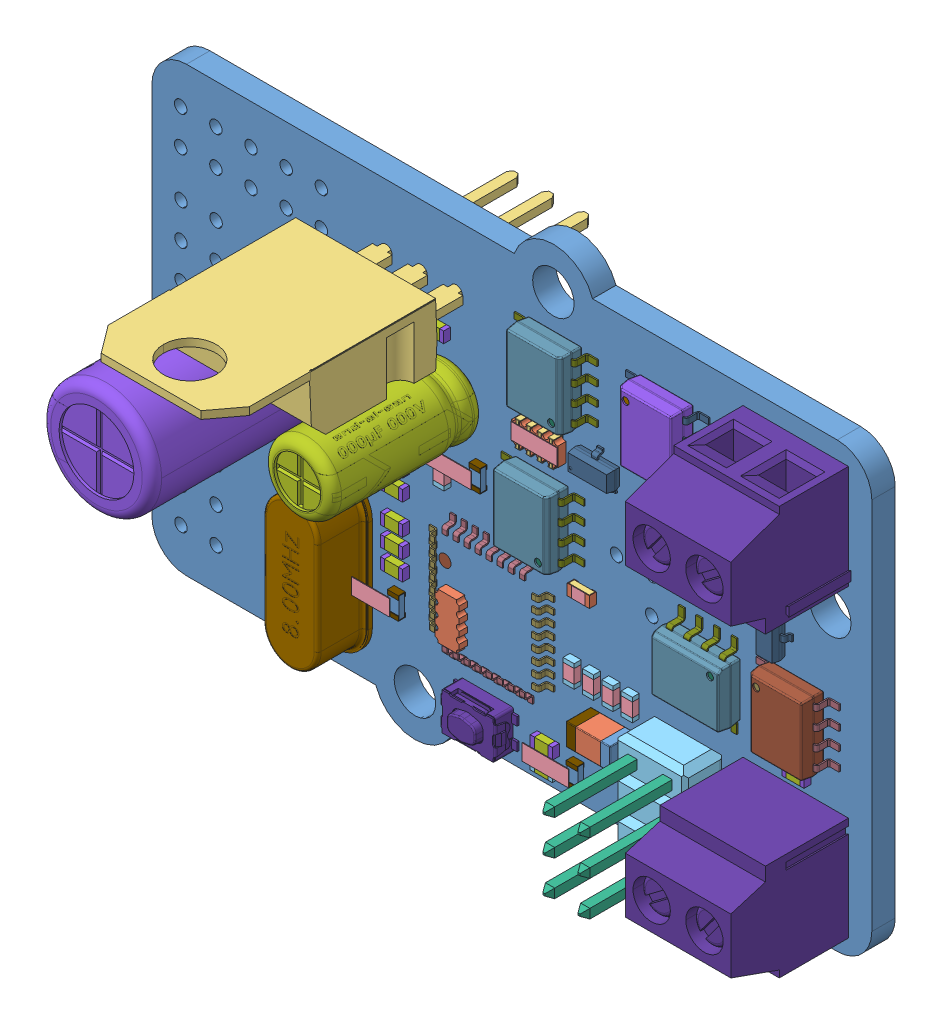
SolidWorks assembly DMotor_PCB v2.8, configuration По умолчанию. Lengths in mm.
Overall size (52 36 28.9).
344 component instances, 44 part files, 0 mates.
Components (placement in the parent):
- DMotor_PCB v2.8.step-1: DMotor_PCB v2.8.step [По умолчанию] at origin size (52 36 28.9)
  - Board.step-1: Board.step [По умолчанию] at origin size (52 36 1.69)
    - Open CASCADE STEP translator 6.8 1.1.1.step-1: Open CASCADE STEP translator 6.8 1.1.1.step [По умолчанию] at (0 0 -1.692) size (52 36 1.69)
  - RN1.step-1: RN1.step [По умолчанию] at origin size (3.35 1.85 0.7)
    - 5778449216.step-1: 5778449216.step [По умолчанию] at (28.3 21.5 0) x (0 1 0) z (0 0 1) size (1.85 3.35 0.7)
      - body.step-1: body.step [По умолчанию] at (-0.875 -1.675 0) size (1.75 3.35 0.6)
        - Open_CASCADE_STEP_translator_6.8_25.1.1.step-1: Open_CASCADE_STEP_translator_6.8_25.1.1.step [По умолчанию] at origin size (1.75 3.35 0.6)
      - Mid_Pin.step-1: Mid_Pin.step [По умолчанию] at (-0.875 -1.2 0) size (0.3 0.38 0.7)
        - Open_CASCADE_STEP_translator_6.8_25.3.1.step-1: Open_CASCADE_STEP_translator_6.8_25.3.1.step [По умолчанию] at origin size (0.3 0.38 0.7)
      - Mid_Pin.step-2: Mid_Pin.step [По умолчанию] at (0.875 1.2 0) x (-1 0 0) z (0 0 1) size (0.3 0.38 0.7)
        - Open_CASCADE_STEP_translator_6.8_25.3.1.step-1: Open_CASCADE_STEP_translator_6.8_25.3.1.step [По умолчанию] at origin size (0.3 0.38 0.7)
      - Mid_Pin.step-3: Mid_Pin.step [По умолчанию] at (-0.875 -0.4 0) size (0.3 0.38 0.7)
        - Open_CASCADE_STEP_translator_6.8_25.3.1.step-1: Open_CASCADE_STEP_translator_6.8_25.3.1.step [По умолчанию] at origin size (0.3 0.38 0.7)
      - Mid_Pin.step-4: Mid_Pin.step [По умолчанию] at (0.875 0.4 0) x (-1 0 0) z (0 0 1) size (0.3 0.38 0.7)
        - Open_CASCADE_STEP_translator_6.8_25.3.1.step-1: Open_CASCADE_STEP_translator_6.8_25.3.1.step [По умолчанию] at origin size (0.3 0.38 0.7)
      - Mid_Pin.step-5: Mid_Pin.step [По умолчанию] at (-0.875 0.4 0) size (0.3 0.38 0.7)
        - Open_CASCADE_STEP_translator_6.8_25.3.1.step-1: Open_CASCADE_STEP_translator_6.8_25.3.1.step [По умолчанию] at origin size (0.3 0.38 0.7)
      - Mid_Pin.step-6: Mid_Pin.step [По умолчанию] at (0.875 -0.4 0) x (-1 0 0) z (0 0 1) size (0.3 0.38 0.7)
        - Open_CASCADE_STEP_translator_6.8_25.3.1.step-1: Open_CASCADE_STEP_translator_6.8_25.3.1.step [По умолчанию] at origin size (0.3 0.38 0.7)
      - Mid_Pin.step-7: Mid_Pin.step [По умолчанию] at (-0.875 1.2 0) size (0.3 0.38 0.7)
        - Open_CASCADE_STEP_translator_6.8_25.3.1.step-1: Open_CASCADE_STEP_translator_6.8_25.3.1.step [По умолчанию] at origin size (0.3 0.38 0.7)
      - Mid_Pin.step-8: Mid_Pin.step [По умолчанию] at (0.875 -1.2 0) x (-1 0 0) z (0 0 1) size (0.3 0.38 0.7)
        - Open_CASCADE_STEP_translator_6.8_25.3.1.step-1: Open_CASCADE_STEP_translator_6.8_25.3.1.step [По умолчанию] at origin size (0.3 0.38 0.7)
      - mark.step-1: mark.step [По умолчанию] at (-0.875 -1.675 0) size (1.15 3.35 0.05)
  - ICSP.step-1: ICSP.step [По умолчанию] at origin size (5.08 7.62 12.7)
    - 2x3_TH_Pitch_2_54mm.step-1: 2x3_TH_Pitch_2_54mm.step [По умолчанию] at (38.7601 0.89 0) x (0 1 0) z (1 0 0) size (7.62 12.7 5.08)
      - header2x3.step-1: header2x3.step [По умолчанию] at (0 1.4 0) size (7.62 2.8 5.08)
      - pin.step-1: pin.step [По умолчанию] at (1.29 -3.5 1.29) size (0.67 12.7 0.67)
      - pin.step-2: pin.step [По умолчанию] at (1.29 -3.5 -1.25) size (0.67 12.7 0.67)
      - pin.step-3: pin.step [По умолчанию] at (3.83 -3.5 1.29) size (0.67 12.7 0.67)
      - pin.step-4: pin.step [По умолчанию] at (3.83 -3.5 -1.25) size (0.67 12.7 0.67)
      - pin.step-5: pin.step [По умолчанию] at (6.37 -3.5 1.29) size (0.67 12.7 0.67)
      - pin.step-6: pin.step [По умолчанию] at (6.37 -3.5 -1.25) size (0.67 12.7 0.67)
  - C9.step-1: C9.step [По умолчанию] at origin size (1.6 0.8 0.5)
    - 5928350752.step-1: 5928350752.step [По умолчанию] at (17.8 11.1 0) size (1 0.8 0.5)
      - Extruded.step-1: Extruded.step [По умолчанию] at origin size (1 0.8 0.5)
    - 5928351312.step-1: 5928351312.step [По умолчанию] at (18.45 11.1 0) size (0.3 0.8 0.5)
      - Extruded-0.step-1: Extruded-0.step [По умолчанию] at origin size (0.3 0.8 0.5)
    - 5928351312.step-2: 5928351312.step [По умолчанию] at (17.15 11.1 0) size (0.3 0.8 0.5)
      - Extruded-0.step-1: Extruded-0.step [По умолчанию] at origin size (0.3 0.8 0.5)
  - C11.step-1: C11.step [По умолчанию] at origin size (1.6 0.8 0.5)
    - 5928350752.step-1: 5928350752.step [По умолчанию] at (17.8 8.3 0) size (1 0.8 0.5)
      - Extruded.step-1: Extruded.step [По умолчанию] at origin size (1 0.8 0.5)
    - 5928351312.step-1: 5928351312.step [По умолчанию] at (18.45 8.3 0) size (0.3 0.8 0.5)
      - Extruded-0.step-1: Extruded-0.step [По умолчанию] at origin size (0.3 0.8 0.5)
    - 5928351312.step-2: 5928351312.step [По умолчанию] at (17.15 8.3 0) size (0.3 0.8 0.5)
      - Extruded-0.step-1: Extruded-0.step [По умолчанию] at origin size (0.3 0.8 0.5)
  - Y1.step-1: Y1.step [По умолчанию] at origin size (4.65 11.35 5.59)
    - HC-49S.step-1: HC-49S.step [По умолчанию] at (13.6 6.8251 0) x (0 1 0) z (1 0 0) size (11.35 5.59 4.65)
  - VT2.step-1: VT2.step [По умолчанию] at origin size (2.9 2.3 1)
    - SOT23-3.step-1: SOT23-3.step [По умолчанию] at (31 21.9 0) x (1 0 0) z (0 -1 0) size (2.9 1 2.3)
  - VT1.step-1: VT1.step [По умолчанию] at origin size (2.3 2.9 1)
    - SOT23-3.step-1: SOT23-3.step [По умолчанию] at (45.2 19.5 0) x (0 -1 0) z (-1 0 0) size (2.9 1 2.3)
  - U1.step-1: U1.step [По умолчанию] at origin size (9 9 1.11)
    - 5778452896.step-1: 5778452896.step [По умолчанию] at (24.6 9.05 0) size (9 9 1.11)
      - body.step-1: body.step [По умолчанию] at (-3.5 -3.5 0) size (1.75 3.35 0.6)
        - Open_CASCADE_STEP_translator_6.8_25.1.1.step-1: Open_CASCADE_STEP_translator_6.8_25.1.1.step [По умолчанию] at origin size (1.75 3.35 0.6)
      - Open_CASCADE_STEP_translator_6.8_22.1.step-1: Open_CASCADE_STEP_translator_6.8_22.1.step [По умолчанию] at (-3.5 -3.5 0.001) size (0.89 0.89 0.01)
      - Leader.step-1: Leader.step [По умолчанию] at (-3.5 -2.8 0) x (-1 0 0) z (0 0 1) size (1 0.38 0.68)
      - Leader.step-2: Leader.step [По умолчанию] at (-3.5 -2 0) x (-1 0 0) z (0 0 1) size (1 0.38 0.68)
      - Leader.step-3: Leader.step [По умолчанию] at (-3.5 -1.2 0) x (-1 0 0) z (0 0 1) size (1 0.38 0.68)
      - Leader.step-4: Leader.step [По умолчанию] at (-3.5 -0.4 0) x (-1 0 0) z (0 0 1) size (1 0.38 0.68)
      - Leader.step-5: Leader.step [По умолчанию] at (-3.5 0.4 0) x (-1 0 0) z (0 0 1) size (1 0.38 0.68)
      - Leader.step-6: Leader.step [По умолчанию] at (-3.5 1.2 0) x (-1 0 0) z (0 0 1) size (1 0.38 0.68)
      - Leader.step-7: Leader.step [По умолчанию] at (-3.5 2 0) x (-1 0 0) z (0 0 1) size (1 0.38 0.68)
      - Leader.step-8: Leader.step [По умолчанию] at (-3.5 2.8 0) x (-1 0 0) z (0 0 1) size (1 0.38 0.68)
      - Leader.step-9: Leader.step [По умолчанию] at (3.5 -2.8 0) size (1 0.38 0.68)
      - Leader.step-10: Leader.step [По умолчанию] at (3.5 -2 0) size (1 0.38 0.68)
      - Leader.step-11: Leader.step [По умолчанию] at (3.5 -1.2 0) size (1 0.38 0.68)
      - Leader.step-12: Leader.step [По умолчанию] at (3.5 -0.4 0) size (1 0.38 0.68)
      - Leader.step-13: Leader.step [По умолчанию] at (3.5 0.4 0) size (1 0.38 0.68)
      - Leader.step-14: Leader.step [По умолчанию] at (3.5 1.2 0) size (1 0.38 0.68)
      - Leader.step-15: Leader.step [По умолчанию] at (3.5 2 0) size (1 0.38 0.68)
      - Leader.step-16: Leader.step [По умолчанию] at (3.5 2.8 0) size (1 0.38 0.68)
      - Leader-1.step-1: Leader-1.step [По умолчанию] at (-2.8 -3.5 0) x (0 -1 0) z (0 0 1) size (1 0.38 0.68)
      - Leader-1.step-2: Leader-1.step [По умолчанию] at (-2 -3.5 0) x (0 -1 0) z (0 0 1) size (1 0.38 0.68)
      - Leader-1.step-3: Leader-1.step [По умолчанию] at (-1.2 -3.5 0) x (0 -1 0) z (0 0 1) size (1 0.38 0.68)
      - Leader-1.step-4: Leader-1.step [По умолчанию] at (-0.4 -3.5 0) x (0 -1 0) z (0 0 1) size (1 0.38 0.68)
      - Leader-1.step-5: Leader-1.step [По умолчанию] at (0.4 -3.5 0) x (0 -1 0) z (0 0 1) size (1 0.38 0.68)
      - Leader-1.step-6: Leader-1.step [По умолчанию] at (1.2 -3.5 0) x (0 -1 0) z (0 0 1) size (1 0.38 0.68)
      - Leader-1.step-7: Leader-1.step [По умолчанию] at (2 -3.5 0) x (0 -1 0) z (0 0 1) size (1 0.38 0.68)
      - Leader-1.step-8: Leader-1.step [По умолчанию] at (2.8 -3.5 0) x (0 -1 0) z (0 0 1) size (1 0.38 0.68)
      - Leader-1.step-9: Leader-1.step [По умолчанию] at (-2.8 3.5 0) x (0 1 0) z (0 0 1) size (1 0.38 0.68)
      - Leader-1.step-10: Leader-1.step [По умолчанию] at (-2 3.5 0) x (0 1 0) z (0 0 1) size (1 0.38 0.68)
      - Leader-1.step-11: Leader-1.step [По умолчанию] at (-1.2 3.5 0) x (0 1 0) z (0 0 1) size (1 0.38 0.68)
      - Leader-1.step-12: Leader-1.step [По умолчанию] at (-0.4 3.5 0) x (0 1 0) z (0 0 1) size (1 0.38 0.68)
      - Leader-1.step-13: Leader-1.step [По умолчанию] at (0.4 3.5 0) x (0 1 0) z (0 0 1) size (1 0.38 0.68)
      - Leader-1.step-14: Leader-1.step [По умолчанию] at (1.2 3.5 0) x (0 1 0) z (0 0 1) size (1 0.38 0.68)
      - Leader-1.step-15: Leader-1.step [По умолчанию] at (2 3.5 0) x (0 1 0) z (0 0 1) size (1 0.38 0.68)
      - Leader-1.step-16: Leader-1.step [По умолчанию] at (2.8 3.5 0) x (0 1 0) z (0 0 1) size (1 0.38 0.68)
  - U2.step-1: U2.step [По умолчанию] at origin size (6 5.01 1.75)
    - 5778448736.step-1: 5778448736.step [По умолчанию] at (28.3 17.1 0) x (-1 0 0) z (0 0 1) size (6 5 1.75)
      - Body-1.step-1: Body-1.step [По умолчанию] at (-2 -2.5 0) size (4 5 1.65)
        - Open_CASCADE_STEP_translator_6.8_4.2.1.step-1: Open_CASCADE_STEP_translator_6.8_4.2.1.step [По умолчанию] at origin size (4 5 1.65)
      - Open_CASCADE_STEP_translator_6.8_4.1.step-1: Open_CASCADE_STEP_translator_6.8_4.1.step [По умолчанию] at (-2 -2.5 0.001) size (0.51 0.51 0.01)
      - Leader-2.step-1: Leader-2.step [По умолчанию] at (-2 -1.905 0) x (-1 0 0) z (0 0 1) size (1 0.42 0.97)
      - Leader-2.step-2: Leader-2.step [По умолчанию] at (-2 -0.635 0) x (-1 0 0) z (0 0 1) size (1 0.42 0.97)
      - Leader-2.step-3: Leader-2.step [По умолчанию] at (-2 0.635 0) x (-1 0 0) z (0 0 1) size (1 0.42 0.97)
      - Leader-2.step-4: Leader-2.step [По умолчанию] at (-2 1.905 0) x (-1 0 0) z (0 0 1) size (1 0.42 0.97)
      - Leader-2.step-5: Leader-2.step [По умолчанию] at (2 -1.905 0) size (1 0.42 0.97)
      - Leader-2.step-6: Leader-2.step [По умолчанию] at (2 -0.635 0) size (1 0.42 0.97)
      - Leader-2.step-7: Leader-2.step [По умолчанию] at (2 0.635 0) size (1 0.42 0.97)
      - Leader-2.step-8: Leader-2.step [По умолчанию] at (2 1.905 0) size (1 0.42 0.97)
  - RESET.step-1: RESET.step [По умолчанию] at origin size (4.6 2.8 1.94)
    - KMR221GLFS.step-1: KMR221GLFS.step [По умолчанию] at (24.2249 2.1749 0) x (-1 0 0) z (0 1 0) size (4.6 1.94 2.8)
  - R7.step-1: R7.step [По умолчанию] at origin size (3.35 1.75 1.15)
    - 5778454576.step-1: 5778454576.step [По умолчанию] at (23.8 17 0) x (0 1 0) z (0 0 1) size (1.75 3.35 1.15)
      - Terminal.step-1: Terminal.step [По умолчанию] at (-0.8 -0.4 0) size (0.3 0.8 0.5)
        - Open_CASCADE_STEP_translator_6.8_7.2.1.step-1: Open_CASCADE_STEP_translator_6.8_7.2.1.step [По умолчанию] at origin size (0.3 0.8 0.5)
      - Terminal.step-2: Terminal.step [По умолчанию] at (0.8 0.4 0) x (-1 0 0) z (0 0 1) size (0.3 0.8 0.5)
        - Open_CASCADE_STEP_translator_6.8_7.2.1.step-1: Open_CASCADE_STEP_translator_6.8_7.2.1.step [По умолчанию] at origin size (0.3 0.8 0.5)
      - Mid_Body.step-1: Mid_Body.step [По умолчанию] at (-0.8 -0.4 0) size (1.5 0.8 0.4)
      - mark.step-1: mark.step [По умолчанию] at (-0.5 -0.4 0.45) size (1.15 3.35 0.05)
  - R6.step-1: R6.step [По умолчанию] at origin size (1.6 0.8 0.5)
    - 5778452416.step-1: 5778452416.step [По умолчанию] at (31.3 13.4 0) x (1 0 0) z (0 0 1) size (1.6 0.8 0.5)
      - Terminal-1.step-1: Terminal-1.step [По умолчанию] at (-0.8 -0.4 0) size (0.3 0.8 0.5)
        - Open_CASCADE_STEP_translator_6.8_7.2.1-3.step-1: Open_CASCADE_STEP_translator_6.8_7.2.1-3.step [По умолчанию] at origin size (0.3 0.8 0.5)
      - Terminal-1.step-2: Terminal-1.step [По умолчанию] at (0.8 0.4 0) x (-1 0 0) z (0 0 1) size (0.3 0.8 0.5)
        - Open_CASCADE_STEP_translator_6.8_7.2.1-3.step-1: Open_CASCADE_STEP_translator_6.8_7.2.1-3.step [По умолчанию] at origin size (0.3 0.8 0.5)
      - Mid_Body-4.step-1: Mid_Body-4.step [По умолчанию] at (-0.8 -0.4 0) size (1.5 0.8 0.4)
      - Mark-5.step-1: Mark-5.step [По умолчанию] at (-0.5 -0.4 0.45) size (1 0.8 0.05)
  - R5.step-1: R5.step [По умолчанию] at origin size (1.6 0.8 0.5)
    - 5778448016.step-1: 5778448016.step [По умолчанию] at (28.625 1.175 0) x (-1 0 0) z (0 0 1) size (1.6 0.8 0.5)
      - Terminal-2.step-1: Terminal-2.step [По умолчанию] at (-0.8 -0.4 0) size (0.3 0.8 0.5)
        - Open_CASCADE_STEP_translator_6.8_7.2.1-6.step-1: Open_CASCADE_STEP_translator_6.8_7.2.1-6.step [По умолчанию] at origin size (0.3 0.8 0.5)
      - Terminal-2.step-2: Terminal-2.step [По умолчанию] at (0.8 0.4 0) x (-1 0 0) z (0 0 1) size (0.3 0.8 0.5)
        - Open_CASCADE_STEP_translator_6.8_7.2.1-6.step-1: Open_CASCADE_STEP_translator_6.8_7.2.1-6.step [По умолчанию] at origin size (0.3 0.8 0.5)
      - Mid_Body-7.step-1: Mid_Body-7.step [По умолчанию] at (-0.8 -0.4 0) size (1.5 0.8 0.4)
      - Mark-8.step-1: Mark-8.step [По умолчанию] at (-0.5 -0.4 0.45) size (1 0.8 0.05)
  - R4.step-1: R4.step [По умолчанию] at origin size (3.35 1.75 1.15)
    - 5778454576.step-1: 5778454576.step [По умолчанию] at (30.825 1.875 0) x (0 1 0) z (0 0 1) size (1.75 3.35 1.15)
      - Terminal.step-1: Terminal.step [По умолчанию] at (-0.8 -0.4 0) size (0.3 0.8 0.5)
        - Open_CASCADE_STEP_translator_6.8_7.2.1.step-1: Open_CASCADE_STEP_translator_6.8_7.2.1.step [По умолчанию] at origin size (0.3 0.8 0.5)
      - Terminal.step-2: Terminal.step [По умолчанию] at (0.8 0.4 0) x (-1 0 0) z (0 0 1) size (0.3 0.8 0.5)
        - Open_CASCADE_STEP_translator_6.8_7.2.1.step-1: Open_CASCADE_STEP_translator_6.8_7.2.1.step [По умолчанию] at origin size (0.3 0.8 0.5)
      - Mid_Body.step-1: Mid_Body.step [По умолчанию] at (-0.8 -0.4 0) size (1.5 0.8 0.4)
      - mark.step-1: mark.step [По умолчанию] at (-0.5 -0.4 0.45) size (1.15 3.35 0.05)
  - R2.step-1: R2.step [По умолчанию] at origin size (3.35 1.75 1.15)
    - 5778454576.step-1: 5778454576.step [По умолчанию] at (10.025 13.8 0) x (0 1 0) z (0 0 1) size (1.75 3.35 1.15)
      - Terminal.step-1: Terminal.step [По умолчанию] at (-0.8 -0.4 0) size (0.3 0.8 0.5)
        - Open_CASCADE_STEP_translator_6.8_7.2.1.step-1: Open_CASCADE_STEP_translator_6.8_7.2.1.step [По умолчанию] at origin size (0.3 0.8 0.5)
      - Terminal.step-2: Terminal.step [По умолчанию] at (0.8 0.4 0) x (-1 0 0) z (0 0 1) size (0.3 0.8 0.5)
        - Open_CASCADE_STEP_translator_6.8_7.2.1.step-1: Open_CASCADE_STEP_translator_6.8_7.2.1.step [По умолчанию] at origin size (0.3 0.8 0.5)
      - Mid_Body.step-1: Mid_Body.step [По умолчанию] at (-0.8 -0.4 0) size (1.5 0.8 0.4)
      - mark.step-1: mark.step [По умолчанию] at (-0.5 -0.4 0.45) size (1.15 3.35 0.05)
  - R3.step-1: R3.step [По умолчанию] at origin size (3.35 1.75 1.15)
    - 5778454576.step-1: 5778454576.step [По умолчанию] at (17.9 6.1 0) x (0 1 0) z (0 0 1) size (1.75 3.35 1.15)
      - Terminal.step-1: Terminal.step [По умолчанию] at (-0.8 -0.4 0) size (0.3 0.8 0.5)
        - Open_CASCADE_STEP_translator_6.8_7.2.1.step-1: Open_CASCADE_STEP_translator_6.8_7.2.1.step [По умолчанию] at origin size (0.3 0.8 0.5)
      - Terminal.step-2: Terminal.step [По умолчанию] at (0.8 0.4 0) x (-1 0 0) z (0 0 1) size (0.3 0.8 0.5)
        - Open_CASCADE_STEP_translator_6.8_7.2.1.step-1: Open_CASCADE_STEP_translator_6.8_7.2.1.step [По умолчанию] at origin size (0.3 0.8 0.5)
      - Mid_Body.step-1: Mid_Body.step [По умолчанию] at (-0.8 -0.4 0) size (1.5 0.8 0.4)
      - mark.step-1: mark.step [По умолчанию] at (-0.5 -0.4 0.45) size (1.15 3.35 0.05)
  - R1.step-1: R1.step [По умолчанию] at origin size (3.35 1.75 1.15)
    - 5778454576.step-1: 5778454576.step [По умолчанию] at (11.425 13.8 0) x (0 1 0) z (0 0 1) size (1.75 3.35 1.15)
      - Terminal.step-1: Terminal.step [По умолчанию] at (-0.8 -0.4 0) size (0.3 0.8 0.5)
        - Open_CASCADE_STEP_translator_6.8_7.2.1.step-1: Open_CASCADE_STEP_translator_6.8_7.2.1.step [По умолчанию] at origin size (0.3 0.8 0.5)
      - Terminal.step-2: Terminal.step [По умолчанию] at (0.8 0.4 0) x (-1 0 0) z (0 0 1) size (0.3 0.8 0.5)
        - Open_CASCADE_STEP_translator_6.8_7.2.1.step-1: Open_CASCADE_STEP_translator_6.8_7.2.1.step [По умолчанию] at origin size (0.3 0.8 0.5)
      - Mid_Body.step-1: Mid_Body.step [По умолчанию] at (-0.8 -0.4 0) size (1.5 0.8 0.4)
      - mark.step-1: mark.step [По умолчанию] at (-0.5 -0.4 0.45) size (1.15 3.35 0.05)
  - Q4.step-1: Q4.step [По умолчанию] at origin size (6 5 1.75)
    - 5778453696.step-1: 5778453696.step [По умолчанию] at (37.3 26.7 0) size (6 5 1.75)
      - Body-2.step-1: Body-2.step [По умолчанию] at (-2 -2.5 0) size (4 5 1.65)
        - Open_CASCADE_STEP_translator_6.8_4.2.1-9.step-1: Open_CASCADE_STEP_translator_6.8_4.2.1-9.step [По умолчанию] at origin size (4 5 1.65)
      - Open_CASCADE_STEP_translator_6.8_4.1-10.step-1: Open_CASCADE_STEP_translator_6.8_4.1-10.step [По умолчанию] at (-2 -2.5 0.001) size (0.51 0.51 0.01)
      - Leader-11.step-1: Leader-11.step [По умолчанию] at (-2 -1.905 0) x (-1 0 0) z (0 0 1) size (1 0.42 0.97)
      - Leader-11.step-2: Leader-11.step [По умолчанию] at (-2 -0.635 0) x (-1 0 0) z (0 0 1) size (1 0.42 0.97)
      - Leader-11.step-3: Leader-11.step [По умолчанию] at (-2 0.635 0) x (-1 0 0) z (0 0 1) size (1 0.42 0.97)
      - Leader-11.step-4: Leader-11.step [По умолчанию] at (-2 1.905 0) x (-1 0 0) z (0 0 1) size (1 0.42 0.97)
      - Leader-11.step-5: Leader-11.step [По умолчанию] at (2 -1.905 0) size (1 0.42 0.97)
      - Leader-11.step-6: Leader-11.step [По умолчанию] at (2 -0.635 0) size (1 0.42 0.97)
      - Leader-11.step-7: Leader-11.step [По умолчанию] at (2 0.635 0) size (1 0.42 0.97)
      - Leader-11.step-8: Leader-11.step [По умолчанию] at (2 1.905 0) size (1 0.42 0.97)
  - Q3.step-1: Q3.step [По умолчанию] at origin size (6 5.01 1.75)
    - 5778448736.step-1: 5778448736.step [По умолчанию] at (29.25 26.3 0) x (-1 0 0) z (0 0 1) size (6 5 1.75)
      - Body-1.step-1: Body-1.step [По умолчанию] at (-2 -2.5 0) size (4 5 1.65)
        - Open_CASCADE_STEP_translator_6.8_4.2.1.step-1: Open_CASCADE_STEP_translator_6.8_4.2.1.step [По умолчанию] at origin size (4 5 1.65)
      - Open_CASCADE_STEP_translator_6.8_4.1.step-1: Open_CASCADE_STEP_translator_6.8_4.1.step [По умолчанию] at (-2 -2.5 0.001) size (0.51 0.51 0.01)
      - Leader-2.step-1: Leader-2.step [По умолчанию] at (-2 -1.905 0) x (-1 0 0) z (0 0 1) size (1 0.42 0.97)
      - Leader-2.step-2: Leader-2.step [По умолчанию] at (-2 -0.635 0) x (-1 0 0) z (0 0 1) size (1 0.42 0.97)
      - Leader-2.step-3: Leader-2.step [По умолчанию] at (-2 0.635 0) x (-1 0 0) z (0 0 1) size (1 0.42 0.97)
      - Leader-2.step-4: Leader-2.step [По умолчанию] at (-2 1.905 0) x (-1 0 0) z (0 0 1) size (1 0.42 0.97)
      - Leader-2.step-5: Leader-2.step [По умолчанию] at (2 -1.905 0) size (1 0.42 0.97)
      - Leader-2.step-6: Leader-2.step [По умолчанию] at (2 -0.635 0) size (1 0.42 0.97)
      - Leader-2.step-7: Leader-2.step [По умолчанию] at (2 0.635 0) size (1 0.42 0.97)
      - Leader-2.step-8: Leader-2.step [По умолчанию] at (2 1.905 0) size (1 0.42 0.97)
  - Q2.step-1: Q2.step [По умолчанию] at origin size (6 5.01 1.75)
    - 5778447616.step-1: 5778447616.step [По умолчанию] at (46.725 13.495 0) x (1 0 0) z (0 0 1) size (6 5 1.75)
      - Body-3.step-1: Body-3.step [По умолчанию] at (-2 -2.5 0) size (4 5 1.65)
        - Open_CASCADE_STEP_translator_6.8_4.2.1-12.step-1: Open_CASCADE_STEP_translator_6.8_4.2.1-12.step [По умолчанию] at origin size (4 5 1.65)
      - Open_CASCADE_STEP_translator_6.8_4.1-13.step-1: Open_CASCADE_STEP_translator_6.8_4.1-13.step [По умолчанию] at (-2 -2.5 0.001) size (0.51 0.51 0.01)
      - Leader-14.step-1: Leader-14.step [По умолчанию] at (-2 -1.905 0) x (-1 0 0) z (0 0 1) size (1 0.42 0.97)
      - Leader-14.step-2: Leader-14.step [По умолчанию] at (-2 -0.635 0) x (-1 0 0) z (0 0 1) size (1 0.42 0.97)
      - Leader-14.step-3: Leader-14.step [По умолчанию] at (-2 0.635 0) x (-1 0 0) z (0 0 1) size (1 0.42 0.97)
      - Leader-14.step-4: Leader-14.step [По умолчанию] at (-2 1.905 0) x (-1 0 0) z (0 0 1) size (1 0.42 0.97)
      - Leader-14.step-5: Leader-14.step [По умолчанию] at (2 -1.905 0) size (1 0.42 0.97)
      - Leader-14.step-6: Leader-14.step [По умолчанию] at (2 -0.635 0) size (1 0.42 0.97)
      - Leader-14.step-7: Leader-14.step [По умолчанию] at (2 0.635 0) size (1 0.42 0.97)
      - Leader-14.step-8: Leader-14.step [По умолчанию] at (2 1.905 0) size (1 0.42 0.97)
  - Q1.step-1: Q1.step [По умолчанию] at origin size (5.01 6 1.75)
    - 5778450736.step-1: 5778450736.step [По умолчанию] at (40.225 13.0265 0) x (0 -1 0) z (0 0 1) size (6 5 1.75)
      - Body-4.step-1: Body-4.step [По умолчанию] at (-2 -2.5 0) size (4 5 1.65)
        - Open_CASCADE_STEP_translator_6.8_4.2.1-15.step-1: Open_CASCADE_STEP_translator_6.8_4.2.1-15.step [По умолчанию] at origin size (4 5 1.65)
      - Open_CASCADE_STEP_translator_6.8_4.1-16.step-1: Open_CASCADE_STEP_translator_6.8_4.1-16.step [По умолчанию] at (-2 -2.5 0.001) size (0.51 0.51 0.01)
      - Leader-17.step-1: Leader-17.step [По умолчанию] at (-2 -1.905 0) x (-1 0 0) z (0 0 1) size (1 0.42 0.97)
      - Leader-17.step-2: Leader-17.step [По умолчанию] at (-2 -0.635 0) x (-1 0 0) z (0 0 1) size (1 0.42 0.97)
      - Leader-17.step-3: Leader-17.step [По умолчанию] at (-2 0.635 0) x (-1 0 0) z (0 0 1) size (1 0.42 0.97)
      - Leader-17.step-4: Leader-17.step [По умолчанию] at (-2 1.905 0) x (-1 0 0) z (0 0 1) size (1 0.42 0.97)
      - Leader-17.step-5: Leader-17.step [По умолчанию] at (2 -1.905 0) size (1 0.42 0.97)
      - Leader-17.step-6: Leader-17.step [По умолчанию] at (2 -0.635 0) size (1 0.42 0.97)
      - Leader-17.step-7: Leader-17.step [По умолчанию] at (2 0.635 0) size (1 0.42 0.97)
      - Leader-17.step-8: Leader-17.step [По умолчанию] at (2 1.905 0) size (1 0.42 0.97)
  - P3.step-1: P3.step [По умолчанию] at origin size (7.81 7.5 12)
    - KLS2-340-3.81.step-1: KLS2-340-3.81.step [По умолчанию] at (46.5051 27.0001 0) size (7.81 7.5 12)
  - P2.step-1: P2.step [По умолчанию] at origin size (7.81 7.5 12)
    - KLS2-340-3.81.step-1: KLS2-340-3.81.step [По умолчанию] at (46.5049 4.9999 0) x (-1 0 0) z (0 0 1) size (7.81 7.5 12)
  - L3.step-1: L3.step [По умолчанию] at origin size (3.2 1.6 1.8)
    - 5778447296.step-1: 5778447296.step [По умолчанию] at (33.3 5.6 0) x (1 0 0) z (0 0 1) size (3.2 1.6 1.8)
      - Terminal-3.step-1: Terminal-3.step [По умолчанию] at (-1.6 -0.8 0) size (3.2 1.6 1.8)
        - Open_CASCADE_STEP_translator_6.8_9.1.1.step-1: Open_CASCADE_STEP_translator_6.8_9.1.1.step [По умолчанию] at origin size (0.7 1.6 1.8)
        - Open_CASCADE_STEP_translator_6.8_9.1.2.step-1: Open_CASCADE_STEP_translator_6.8_9.1.2.step [По умолчанию] at origin size (0.7 1.6 1.8)
      - Mid_Body-18.step-1: Mid_Body-18.step [По умолчанию] at (-1.6 -0.8 0) size (1.8 1.6 1.8)
        - Open_CASCADE_STEP_translator_6.8_9.2.1.step-1: Open_CASCADE_STEP_translator_6.8_9.2.1.step [По умолчанию] at origin size (1.8 1.6 1.8)
  - DA1.step-1: DA1.step [По умолчанию] at origin size (10.2 4.5 28.9)
    - TO220.step-1: TO220.step [По умолчанию] at (19.4399 30.3489 4) x (1 0 0) z (0 -1 0) size (10.2 28.9 4.5)
  - C21.step-1: C21.step [По умолчанию] at origin size (0.8 1.6 0.5)
    - 5928349552.step-1: 5928349552.step [По умолчанию] at (41.7 26.9 0) size (0.8 1 0.5)
      - Extruded-19.step-1: Extruded-19.step [По умолчанию] at origin size (0.8 1 0.5)
    - 5928349232.step-1: 5928349232.step [По умолчанию] at (41.7 26.25 0) size (0.8 0.3 0.5)
      - Extruded-20.step-1: Extruded-20.step [По умолчанию] at origin size (0.8 0.3 0.5)
    - 5928349232.step-2: 5928349232.step [По умолчанию] at (41.7 27.55 0) size (0.8 0.3 0.5)
      - Extruded-20.step-1: Extruded-20.step [По умолчанию] at origin size (0.8 0.3 0.5)
  - C20.step-1: C20.step [По умолчанию] at origin size (1.6 0.8 0.5)
    - 5928351312.step-1: 5928351312.step [По умолчанию] at (46.15 9.9 0) size (0.3 0.8 0.5)
      - Extruded-0.step-1: Extruded-0.step [По умолчанию] at origin size (0.3 0.8 0.5)
    - 5928351312.step-2: 5928351312.step [По умолчанию] at (47.45 9.9 0) size (0.3 0.8 0.5)
      - Extruded-0.step-1: Extruded-0.step [По умолчанию] at origin size (0.3 0.8 0.5)
    - 5928350752.step-1: 5928350752.step [По умолчанию] at (46.8 9.9 0) size (1 0.8 0.5)
      - Extruded.step-1: Extruded.step [По умолчанию] at origin size (1 0.8 0.5)
  - C19.step-1: C19.step [По умолчанию] at origin size (0.8 1.6 0.5)
    - 5928349552.step-1: 5928349552.step [По умолчанию] at (21.2 15.9 0) size (0.8 1 0.5)
      - Extruded-19.step-1: Extruded-19.step [По умолчанию] at origin size (0.8 1 0.5)
    - 5928349232.step-1: 5928349232.step [По умолчанию] at (21.2 16.55 0) size (0.8 0.3 0.5)
      - Extruded-20.step-1: Extruded-20.step [По умолчанию] at origin size (0.8 0.3 0.5)
    - 5928349232.step-2: 5928349232.step [По умолчанию] at (21.2 15.25 0) size (0.8 0.3 0.5)
      - Extruded-20.step-1: Extruded-20.step [По умолчанию] at origin size (0.8 0.3 0.5)
  - C18.step-1: C18.step [По умолчанию] at origin size (1.6 0.8 0.5)
    - 5928351312.step-1: 5928351312.step [По умолчанию] at (27.975 2.575 0) size (0.3 0.8 0.5)
      - Extruded-0.step-1: Extruded-0.step [По умолчанию] at origin size (0.3 0.8 0.5)
    - 5928351312.step-2: 5928351312.step [По умолчанию] at (29.275 2.575 0) size (0.3 0.8 0.5)
      - Extruded-0.step-1: Extruded-0.step [По умолчанию] at origin size (0.3 0.8 0.5)
    - 5928350752.step-1: 5928350752.step [По умолчанию] at (28.625 2.575 0) size (1 0.8 0.5)
      - Extruded.step-1: Extruded.step [По умолчанию] at origin size (1 0.8 0.5)
  - C17.step-1: C17.step [По умолчанию] at origin size (0.8 1.6 0.5)
    - 5928349552.step-1: 5928349552.step [По умолчанию] at (10.3 5.2 0) size (0.8 1 0.5)
      - Extruded-19.step-1: Extruded-19.step [По умолчанию] at origin size (0.8 1 0.5)
    - 5928349232.step-1: 5928349232.step [По умолчанию] at (10.3 4.55 0) size (0.8 0.3 0.5)
      - Extruded-20.step-1: Extruded-20.step [По умолчанию] at origin size (0.8 0.3 0.5)
    - 5928349232.step-2: 5928349232.step [По умолчанию] at (10.3 5.85 0) size (0.8 0.3 0.5)
      - Extruded-20.step-1: Extruded-20.step [По умолчанию] at origin size (0.8 0.3 0.5)
  - C16.step-1: C16.step [По умолчанию] at origin size (0.8 1.6 0.5)
    - 5928349552.step-1: 5928349552.step [По умолчанию] at (10.3 8.2 0) size (0.8 1 0.5)
      - Extruded-19.step-1: Extruded-19.step [По умолчанию] at origin size (0.8 1 0.5)
    - 5928349232.step-1: 5928349232.step [По умолчанию] at (10.3 7.55 0) size (0.8 0.3 0.5)
      - Extruded-20.step-1: Extruded-20.step [По умолчанию] at origin size (0.8 0.3 0.5)
    - 5928349232.step-2: 5928349232.step [По умолчанию] at (10.3 8.85 0) size (0.8 0.3 0.5)
      - Extruded-20.step-1: Extruded-20.step [По умолчанию] at origin size (0.8 0.3 0.5)
  - C15.step-1: C15.step [По умолчанию] at origin size (0.8 1.6 0.5)
    - 5928349552.step-1: 5928349552.step [По умолчанию] at (30.6 8.2 0) size (0.8 1 0.5)
      - Extruded-19.step-1: Extruded-19.step [По умолчанию] at origin size (0.8 1 0.5)
    - 5928349232.step-1: 5928349232.step [По умолчанию] at (30.6 7.55 0) size (0.8 0.3 0.5)
      - Extruded-20.step-1: Extruded-20.step [По умолчанию] at origin size (0.8 0.3 0.5)
    - 5928349232.step-2: 5928349232.step [По умолчанию] at (30.6 8.85 0) size (0.8 0.3 0.5)
      - Extruded-20.step-1: Extruded-20.step [По умолчанию] at origin size (0.8 0.3 0.5)
  - C14.step-1: C14.step [По умолчанию] at origin size (0.8 1.6 0.5)
    - 5928349552.step-1: 5928349552.step [По умолчанию] at (32 8.2 0) size (0.8 1 0.5)
      - Extruded-19.step-1: Extruded-19.step [По умолчанию] at origin size (0.8 1 0.5)
    - 5928349232.step-1: 5928349232.step [По умолчанию] at (32 7.55 0) size (0.8 0.3 0.5)
      - Extruded-20.step-1: Extruded-20.step [По умолчанию] at origin size (0.8 0.3 0.5)
    - 5928349232.step-2: 5928349232.step [По умолчанию] at (32 8.85 0) size (0.8 0.3 0.5)
      - Extruded-20.step-1: Extruded-20.step [По умолчанию] at origin size (0.8 0.3 0.5)
  - C13.step-1: C13.step [По умолчанию] at origin size (0.8 1.6 0.5)
    - 5928349552.step-1: 5928349552.step [По умолчанию] at (33.4 8.2 0) size (0.8 1 0.5)
      - Extruded-19.step-1: Extruded-19.step [По умолчанию] at origin size (0.8 1 0.5)
    - 5928349232.step-1: 5928349232.step [По умолчанию] at (33.4 7.55 0) size (0.8 0.3 0.5)
      - Extruded-20.step-1: Extruded-20.step [По умолчанию] at origin size (0.8 0.3 0.5)
    - 5928349232.step-2: 5928349232.step [По умолчанию] at (33.4 8.85 0) size (0.8 0.3 0.5)
      - Extruded-20.step-1: Extruded-20.step [По умолчанию] at origin size (0.8 0.3 0.5)
  - C12.step-1: C12.step [По умолчанию] at origin size (0.8 1.6 0.5)
    - 5928349552.step-1: 5928349552.step [По умолчанию] at (34.8 8.2 0) size (0.8 1 0.5)
      - Extruded-19.step-1: Extruded-19.step [По умолчанию] at origin size (0.8 1 0.5)
    - 5928349232.step-1: 5928349232.step [По умолчанию] at (34.8 7.55 0) size (0.8 0.3 0.5)
      - Extruded-20.step-1: Extruded-20.step [По умолчанию] at origin size (0.8 0.3 0.5)
    - 5928349232.step-2: 5928349232.step [По умолчанию] at (34.8 8.85 0) size (0.8 0.3 0.5)
      - Extruded-20.step-1: Extruded-20.step [По умолчанию] at origin size (0.8 0.3 0.5)
  - C10.step-1: C10.step [По умолчанию] at origin size (1.6 0.8 0.5)
    - 5928350752.step-1: 5928350752.step [По умолчанию] at (17.8 9.7 0) size (1 0.8 0.5)
      - Extruded.step-1: Extruded.step [По умолчанию] at origin size (1 0.8 0.5)
    - 5928351312.step-1: 5928351312.step [По умолчанию] at (18.45 9.7 0) size (0.3 0.8 0.5)
      - Extruded-0.step-1: Extruded-0.step [По умолчанию] at origin size (0.3 0.8 0.5)
    - 5928351312.step-2: 5928351312.step [По умолчанию] at (17.15 9.7 0) size (0.3 0.8 0.5)
      - Extruded-0.step-1: Extruded-0.step [По умолчанию] at origin size (0.3 0.8 0.5)
  - C8.step-1: C8.step [По умолчанию] at origin size (1.6 0.8 0.5)
    - 5928350752.step-1: 5928350752.step [По умолчанию] at (17.8 13.3 0) size (1 0.8 0.5)
      - Extruded.step-1: Extruded.step [По умолчанию] at origin size (1 0.8 0.5)
    - 5928351312.step-1: 5928351312.step [По умолчанию] at (18.45 13.3 0) size (0.3 0.8 0.5)
      - Extruded-0.step-1: Extruded-0.step [По умолчанию] at origin size (0.3 0.8 0.5)
    - 5928351312.step-2: 5928351312.step [По умолчанию] at (17.15 13.3 0) size (0.3 0.8 0.5)
      - Extruded-0.step-1: Extruded-0.step [По умолчанию] at origin size (0.3 0.8 0.5)
  - C7.step-1: C7.step [По умолчанию] at origin size (1.6 0.8 0.5)
    - 5928350752.step-1: 5928350752.step [По умолчанию] at (17.8 14.8 0) size (1 0.8 0.5)
      - Extruded.step-1: Extruded.step [По умолчанию] at origin size (1 0.8 0.5)
    - 5928351312.step-1: 5928351312.step [По умолчанию] at (18.45 14.8 0) size (0.3 0.8 0.5)
      - Extruded-0.step-1: Extruded-0.step [По умолчанию] at origin size (0.3 0.8 0.5)
    - 5928351312.step-2: 5928351312.step [По умолчанию] at (17.15 14.8 0) size (0.3 0.8 0.5)
      - Extruded-0.step-1: Extruded-0.step [По умолчанию] at origin size (0.3 0.8 0.5)
  - C6.step-1: C6.step [По умолчанию] at origin size (3.7 2.93 2.03)
    - TANT-B.step-1: TANT-B.step [По умолчанию] at (17.8999 17.1999 0) x (-1 0 0) z (0 0 1) size (3.7 2.93 2.03)
  - C5.step-1: C5.step [По умолчанию] at origin size (5.05 5.02 13.81)
    - Cap-EL(5x11-2)T.step-1: Cap-EL(5x11-2)T.step [По умолчанию] at (21.8001 21.2001 0.3) x (1 0 0) z (0 0 1) size (5.05 5.02 13.81)
  - C4.step-1: C4.step [По умолчанию] at origin size (1.6 0.8 0.5)
    - 5928350752.step-1: 5928350752.step [По умолчанию] at (20.775 24.7 0) size (1 0.8 0.5)
      - Extruded.step-1: Extruded.step [По умолчанию] at origin size (1 0.8 0.5)
    - 5928351312.step-1: 5928351312.step [По умолчанию] at (21.425 24.7 0) size (0.3 0.8 0.5)
      - Extruded-0.step-1: Extruded-0.step [По умолчанию] at origin size (0.3 0.8 0.5)
    - 5928351312.step-2: 5928351312.step [По умолчанию] at (20.125 24.7 0) size (0.3 0.8 0.5)
      - Extruded-0.step-1: Extruded-0.step [По умолчанию] at origin size (0.3 0.8 0.5)
  - C3.step-1: C3.step [По умолчанию] at origin size (1.6 0.8 0.5)
    - 5928350752.step-1: 5928350752.step [По умолчанию] at (17.775 24.7 0) size (1 0.8 0.5)
      - Extruded.step-1: Extruded.step [По умолчанию] at origin size (1 0.8 0.5)
    - 5928351312.step-1: 5928351312.step [По умолчанию] at (17.125 24.7 0) size (0.3 0.8 0.5)
      - Extruded-0.step-1: Extruded-0.step [По умолчанию] at origin size (0.3 0.8 0.5)
    - 5928351312.step-2: 5928351312.step [По умолчанию] at (18.425 24.7 0) size (0.3 0.8 0.5)
      - Extruded-0.step-1: Extruded-0.step [По умолчанию] at origin size (0.3 0.8 0.5)
  - C2.step-1: C2.step [По умолчанию] at origin size (1.6 0.8 0.5)
    - 5928350752.step-1: 5928350752.step [По умолчанию] at (17.8 23.2 0) size (1 0.8 0.5)
      - Extruded.step-1: Extruded.step [По умолчанию] at origin size (1 0.8 0.5)
    - 5928351312.step-1: 5928351312.step [По умолчанию] at (17.15 23.2 0) size (0.3 0.8 0.5)
      - Extruded-0.step-1: Extruded-0.step [По умолчанию] at origin size (0.3 0.8 0.5)
    - 5928351312.step-2: 5928351312.step [По умолчанию] at (18.45 23.2 0) size (0.3 0.8 0.5)
      - Extruded-0.step-1: Extruded-0.step [По умолчанию] at origin size (0.3 0.8 0.5)
  - C1.step-1: C1.step [По умолчанию] at origin size (8.01 8 19.31)
    - Cap-EL(8x16-3_5).step-1: Cap-EL(8x16-3_5).step [По умолчанию] at (12.4999 21 0.5) x (-1 0 0) z (0 0 1) size (8.01 8 19.31)
